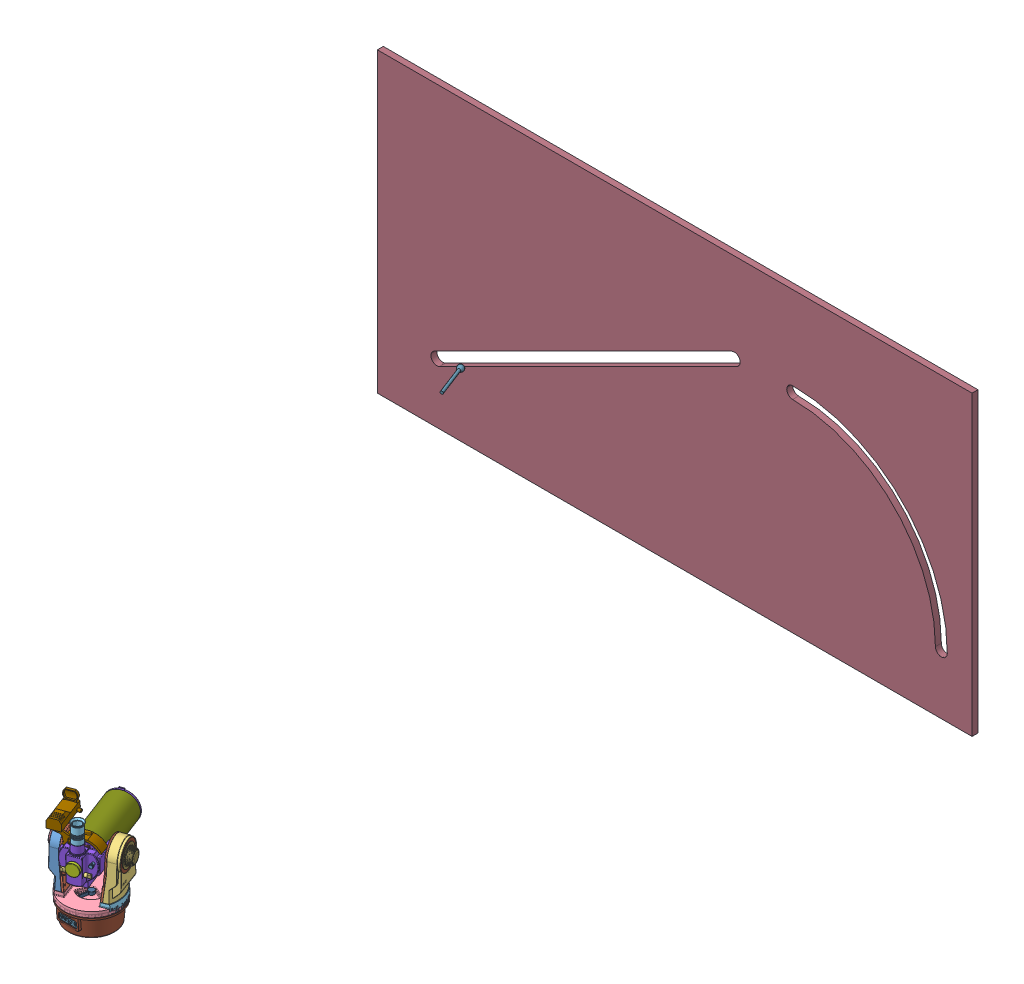
SolidWorks assembly meade, configuration Défaut. Lengths in mm.
Overall size (2000 1013.54 2177.52).
169 component instances, 90 part files, 14 mates.
Components (placement in the parent):
- fourche-1: fourche [Défaut] at (-625.4389 13.0791 -499.8104) x (-0.957342 -0.017413 0.288434) z (-0.288497 0.001172 -0.95748) size (198.85 238.33 188.61)
  - branche equilibrage-1: branche equilibrage [Défaut] at (-444.0293 45.9192 -837.0232) x (0.999848 0.017413 0.00001) z (0.00001 -0.001172 0.999999) size (42.16 177.75 110.07)
  - Plaque carter équilibrage-1: Plaque carter équilibrage [Défaut] at (-443.0317 45.9366 -837.0903) x (0.999848 0.017413 0.00001) z (0.00001 -0.001172 0.999999) size (27.56 165.18 109.18)
  - Plaque carter équilibrage-2: Plaque carter équilibrage [Défaut] at (-468.0617 45.0668 -480.7137) x (-0.999848 -0.017413 -0.00001) z (-0.00001 0.001172 -0.999999) size (27.56 165.18 109.18)
  - branche motorisée-1: branche motorisée [Défaut] at (-441.716 45.9434 -837.1795) x (0.999848 0.017413 0.00001) z (0.00001 -0.001172 0.999999) size (49.59 177.72 110.04)
  - PIED DE fourche-1: PIED DE fourche [Défaut] at (-454.4692 -14.4541 -658.8869) x (0.999848 0.017413 0.00001) z (0.00001 -0.001172 0.999999) size (191.94 35.1 188.57)
    - Pied de fourche-1: Pied de fourche [Défaut] at (12.1809 59.9857 -178.2534) size (191.94 35.1 188.57)
    - Pied de fourche1-1: Pied de fourche1 [Défaut] at (-12.1809 59.9857 178.0188) x (-1 0 0) z (0 0 -1) size (54.8 35.1 115.86)
  - rondelle vis m8_50-1: rondelle vis m8_50 [Défaut] at (-454.2843 -25.0712 -659.0167) x (0.997592 0.017452 -0.067129) z (0.017413 -0.999848 -0.001172) size (26.8 26.16 7)
  - VisHM8_50-1: VisHM8_50 [Défaut] at (-454.3818 -19.4721 -659.0102) x (0.997592 0.017452 -0.067129) z (0.017413 -0.999848 -0.001172) size (12.6 14.55 55.47)
  - limiteur de couple embase-1: limiteur de couple embase [Défaut] at (-453.5008 -70.0544 -659.0694) x (0.06714 0 0.997744) z (-0.997592 -0.017452 0.067129) size (25.3 5 25.3)
  - Roue à denture hélicoïdale m=0,5 Z=60-1: Roue à denture hélicoïdale m=0,5 Z=60 [Défaut] at (-453.6431 -61.8856 -659.0599) x (0.201032 0.002353 0.979582) z (-0.017413 0.999848 0.001172) size (31.07 31.07 6.34)
  - Levier de débrayage-1: Levier de débrayage [Défaut] at (-491.4971 43.1006 -833.8173) x (0.963244 0.01709 -0.268082) z (0.268062 0.003539 0.963395) size (36.12 10 38.96)
  - plateau-1: plateau [Défaut] at (-454.3861 -19.2221 -659.0099) x (-0.997592 -0.017452 0.067129) z (0.017413 -0.999848 -0.001172) size (170 170 47)
  - EcrouHM 20-2: EcrouHM 20 [Défaut] at (-453.9456 -44.5183 -659.0395) x (0.06714 0 0.997744) z (-0.017413 0.999848 0.001172) size (30 34.64 12)
  - motoreducteur fourche-1: motoreducteur fourche [Défaut] at (-542.1299 45.8782 -641.824) x (0.06714 0 0.997744) z (0.997592 0.017452 -0.067129) size (70.5 139.71 33.06)
    - rep. 01 pignon arbre moteur + disque-1: rep. 01 pignon arbre moteur + disque [Défaut] at (0 -0.36 0) size (19 10.8 19)
    - rep. 02-03 roue Z56-1: rep. 02-03 roue Z56 [Défaut] at (0.8779 -0.6486 0.8082) x (0.995701 0 0.092628) z (-0.092628 0 0.995701) size (28.76 10.95 28.76)
    - rep. 08-09 roue inter-1: rep. 08-09 roue inter [Défaut] at (-0.15 -0.2381 0) x (1 0 0) z (0 0 1) size (12.96 5.74 12.96)
    - rep. 06-07 roue inter-1: rep. 06-07 roue inter [Défaut] at (-0.15 -0.0981 0) x (1 0 0) z (0 0 1) size (13 5.74 13)
    - rep. 04-05 roue inter-1: rep. 04-05 roue inter [Défaut] at (-21.6079 -0.6386 5.1059) x (0.907401 0 -0.420265) z (0.420265 0 0.907401) size (13 5.74 13)
    - bati-1: bati [Défaut] at (103.3128 129.885 -87.3106) size (70.5 138.91 24)
      - Axe Rep19bis-1: Axe Rep19bis [Défaut] at (-92.1856 -130.245 98.2871) x (-0.137137 0 0.990552) z (-0.990552 0 -0.137137) size (3 14 3)
      - moteur-1: moteur [Défaut] at (-103.3128 -129.885 87.3106) size (18 46.5 24)
      - axe-1: axe [Défaut] at (-111.605 -120.0821 97.7106) x (0.934599 0 -0.355704) z (0 -1 0) size (3 3 39)
      - bati2-1: bati2 [Défaut] at (-77.4849 -277.8736 138.6581) x (1 0 0) z (0 0 -1) size (17.4 55.11 17.4)
        - rondelle alu-1: rondelle alu [Défaut] at (-55.9783 -35.2009 30.6529) size (17.4 2.5 17.4)
        - Rondelle M6_1-1: Rondelle M6_1 [Défaut] at (-55.9783 -35.2009 30.6529) size (16.67 2.55 16.67)
        - rondelle alu_1-1: rondelle alu_1 [Défaut] at (-55.9783 -35.2009 30.6529) size (17.4 2.5 17.4)
        - Entretoise_1-1: Entretoise_1 [Défaut] at (-55.9783 -35.2009 30.6529) size (16.5 6 16.5)
        - Entretoise-1: Entretoise [Défaut] at (-55.9783 -35.2009 30.6529) size (16.5 6 16.5)
        - Rondelle M6-1: Rondelle M6 [Défaut] at (-55.9783 -35.2009 30.6529) size (16.67 2.55 16.67)
        - rep. 16 Ecrou M6-1: rep. 16 Ecrou M6 [Défaut] at (18.5294 -120.4752 48.0628) x (-0.896454 0 -0.443136) z (-0.443136 0 0.896454) size (12.68 6 11.39)
      - corps1-1: corps1 [Défaut] at (-126.5989 -147.7633 97.7106) size (62.7 74.5 12)
      - corps2-1: corps2 [Défaut] at (-126.5989 -147.7633 85.7106) size (62.7 50 12)
      - châpe en alu-1: châpe en alu [Défaut] at (-133.4632 -157.3984 87.2051) size (33.3 38 19.61)
    - vis-1: vis [Défaut] at (7.3554 -71.4832 9.6533) x (1 0 0) z (0 1 0) size (33.09 33.06 82.71)
      - Vis san fin m=0,5 - 1 filet(s)-2: Vis san fin m=0,5 - 1 filet(s) [Défaut] at (-0.6479 -0.6412 0.3804) x (0.7262 -0.687484 0) z (0 0 1) size (8.16 8.16 68.9)
      - rep12-4: rep12 [Défaut] at (-11.6724 36.0347 43.7266) x (0.537117 -0.843508 0) z (-0.843508 -0.537117 0) size (23.91 29.81 24)
    - engrenage-1: engrenage [Défaut] at (-45.9983 -125.8694 31.0757) x (-0.919401 0 0.393321) z (0.393321 0 0.919401) size (12.99 17.44 12.99)
      - rep.11SLDPRT-1: rep.11SLDPRT [Défaut] at (-64.557 -106.8565 -14.5787) size (9.52 16 9.52)
      - rep. yacine-1: rep. yacine [Défaut] at (-64.557 -106.8565 -14.5787) size (12.99 1.44 12.99)
    - Vis à tête cylindrique à six pans creux Chc M2,5 - 8-1: Vis à tête cylindrique à six pans creux Chc M2,5 - 8 [Défaut] at (6.7074 -20.6971 10.2945) x (0.636786 0 0.771041) z (0 -1 0) size (4.2 4.2 10.57)
    - joint 9 5 emb-1: joint 9 5 emb [Défaut] at (6.7074 -89.1506 10.2945) size (13.5 2 13.5)
    - joint 9 5 emb-2: joint 9 5 emb [Défaut] at (6.7074 -53.1506 10.2945) size (13.5 2 13.5)
  - Vis sans tête à six pans creux à bout cuvette M3 - 3-1: Vis sans tête à six pans creux à bout cuvette M3 - 3 [Réaliste] at (-445.1418 -17.1499 -659.6319) x (-0.019293 -0.859815 -0.51024) z (0.066624 -0.510307 0.857408) size (3.03 3.08 3.04)
  - Vis à tête cylindrique bombée cruciforme type H M3 - 10-1: Vis à tête cylindrique bombée cruciforme type H M3 - 10 [Filetage Réaliste] at (-521.841 56.7793 -695.504) x (-0.997592 -0.017452 0.067129) z (-0.0364 0.955572 -0.292501) size (12.58 5.6 5.6)
  - Vis à tête cylindrique bombée cruciforme type H M3 - 10-2: Vis à tête cylindrique bombée cruciforme type H M3 - 10 [Filetage Réaliste] at (-508.9533 16.8988 -611.179) x (-0.997592 -0.017452 0.067129) z (-0.040277 -0.642181 -0.765494) size (12.58 5.6 5.6)
  - Vis à tête cylindrique bombée cruciforme type H M3 - 10-3: Vis à tête cylindrique bombée cruciforme type H M3 - 10 [Filetage Réaliste] at (-514.8616 16.8988 -698.9804) x (-0.997592 -0.017452 0.067129) z (-0.068087 0.06176 -0.995766) size (12.58 5.6 5.6)
  - Vis à tête cylindrique bombée cruciforme type H M3 - 10-4: Vis à tête cylindrique bombée cruciforme type H M3 - 10 [Filetage Réaliste] at (-521.2936 154.7556 -654.4481) x (-0.997592 -0.017452 0.067129) z (-0.06714 0 -0.997744) size (12.58 5.6 5.6)
  - Vis à tête cylindrique bombée cruciforme type H M3 - 10-5: Vis à tête cylindrique bombée cruciforme type H M3 - 10 [Filetage Réaliste] at (-516.3356 56.7793 -613.689) x (-0.997592 -0.017452 0.067129) z (-0.06714 0 -0.997744) size (12.58 5.6 5.6)
  - Vis à tête cylindrique bombée cruciforme type H M3 - 10-7: Vis à tête cylindrique bombée cruciforme type H M3 - 10 [Filetage Réaliste] at (-393.6444 157.0051 -663.0973) x (0.997592 0.017452 -0.067129) z (0.06714 0 0.997744) size (12.58 5.6 5.6)
  - Vis à tête cylindrique bombée cruciforme type H M3 - 10-8: Vis à tête cylindrique bombée cruciforme type H M3 - 10 [Filetage Réaliste] at (-401.1787 18.9039 -706.6898) x (0.997592 0.017452 -0.067129) z (0.06714 0 0.997744) size (12.58 5.6 5.6)
  - Vis à tête cylindrique bombée cruciforme type H M3 - 10-10: Vis à tête cylindrique bombée cruciforme type H M3 - 10 [Filetage Réaliste] at (-395.1895 59.0113 -704.086) x (0.997592 0.017452 -0.067129) z (0.06714 0 0.997744) size (12.58 5.6 5.6)
  - Vis à tête cylindrique fendue CS M4 - 10-1: Vis à tête cylindrique fendue CS M4 - 10 [Défaut] at (-539.7157 125.5672 -628.3483) x (0.067415 -0.016315 0.997592) z (-0.997592 -0.017452 0.067129) size (7 7 10.62)
  - Vis à tête cylindrique fendue CS M4 - 10-2: Vis à tête cylindrique fendue CS M4 - 10 [Défaut] at (-538.2089 116.0774 -615.8713) x (0.067415 -0.016315 0.997592) z (-0.997592 -0.017452 0.067129) size (7 7 10.62)
  - Vis à tête cylindrique fendue CS M4 - 10-3: Vis à tête cylindrique fendue CS M4 - 10 [Défaut] at (-539.3849 106.5701 -628.3705) x (0.067415 -0.016315 0.997592) z (-0.997592 -0.017452 0.067129) size (7 7 10.62)
  - Vis à tête cylindrique bombée cruciforme type H M3 - 12-2: Vis à tête cylindrique bombée cruciforme type H M3 - 12 [Filetage Réaliste] at (-395.2704 18.9039 -618.8883) x (0.997592 0.017452 -0.067129) z (0.067129 0.000586 0.997744) size (14.59 5.6 5.6)
  - Vis à tête cylindrique bombée cruciforme type H M3 - 12-3: Vis à tête cylindrique bombée cruciforme type H M3 - 12 [Filetage Réaliste] at (-389.684 59.0113 -622.271) x (0.997592 0.017452 -0.067129) z (0.068185 -0.42423 0.902984) size (14.59 5.6 5.6)
  - Vis à tête cylindrique bombée cruciforme type H M3 - 25-1: Vis à tête cylindrique bombée cruciforme type H M3 - 25 [Filetage Réaliste] at (-516.5693 58.6063 -628.1014) x (-0.997592 -0.017452 0.067129) z (-0.067129 0.486457 -0.871122) size (32.61 5.6 5.6)
  - Vis à tête cylindrique bombée cruciforme type H M3 - 25-2: Vis à tête cylindrique bombée cruciforme type H M3 - 25 [Filetage Réaliste] at (-520.3322 72.7741 -680.3366) x (-0.997592 -0.017452 0.067129) z (-0.067129 0.486457 -0.871122) size (32.61 5.6 5.6)
  - Vis à tête cylindrique bombée cruciforme type H M3 - 25-3: Vis à tête cylindrique bombée cruciforme type H M3 - 25 [Filetage Réaliste] at (-519.8272 43.7786 -680.3706) x (-0.997592 -0.017452 0.067129) z (0.067053 0.00493 0.997737) size (32.61 5.6 5.6)
  - Vis à tête cylindrique bombée cruciforme type H M3 - 20-1: Vis à tête cylindrique bombée cruciforme type H M3 - 20 [Filetage Réaliste] at (-531.1265 -25.9655 -653.8459) x (-0.017413 0.999848 0.001172) z (0.998816 0.017342 0.045444) size (22.61 5.6 5.6)
  - Vis à tête cylindrique bombée cruciforme type H M3 - 20-2: Vis à tête cylindrique bombée cruciforme type H M3 - 20 [Filetage Réaliste] at (-512.8439 -25.695 -612.9812) x (-0.017413 0.999848 0.001172) z (0.998816 0.017342 0.045444) size (22.61 5.6 5.6)
  - Vis à tête cylindrique bombée cruciforme type H M3 - 20-3: Vis à tête cylindrique bombée cruciforme type H M3 - 20 [Filetage Réaliste] at (-517.7505 -25.6821 -696.841) x (-0.017413 0.999848 0.001172) z (0.998816 0.017342 0.045444) size (22.61 5.6 5.6)
  - Vis à tête cylindrique bombée cruciforme type H M3 - 20-4: Vis à tête cylindrique bombée cruciforme type H M3 - 20 [Filetage Réaliste] at (-395.7403 -23.5476 -705.0512) x (-0.017413 0.999848 0.001172) z (0.998816 0.017342 0.045444) size (22.61 5.6 5.6)
  - Vis à tête cylindrique bombée cruciforme type H M3 - 20-5: Vis à tête cylindrique bombée cruciforme type H M3 - 20 [Filetage Réaliste] at (-377.4577 -23.2771 -664.1865) x (-0.017413 0.999848 0.001172) z (0.998816 0.017342 0.045444) size (22.61 5.6 5.6)
  - Vis à tête cylindrique bombée cruciforme type H M3 - 20-6: Vis à tête cylindrique bombée cruciforme type H M3 - 20 [Filetage Réaliste] at (-390.8337 -23.5604 -621.1914) x (-0.017413 0.999848 0.001172) z (0.998816 0.017342 0.045444) size (22.61 5.6 5.6)
- tube-1: tube [Défaut] at (-0.2356 70.625 -0.6263) x (-0.935954 0 0.352121) z (-0.352104 0.009923 -0.935908) size (229.47 195.18 484.9)
  - Capuchon port photo-2: Capuchon port photo [Défaut] at (20.0265 52.1414 -183.8549) x (0.753442 -0.654583 0.06202) z (-0.29492 -0.252137 0.921656) size (39.95 39.82 23.78)
  - support objectif-2: support objectif [Défaut] at (0 67.5 -76) size (179.88 130.77 134.7)
  - Palier d'embrayage-2: Palier d'embrayage [Défaut] at (24.7034 252.6163 -72.3954) x (0.997744 -0.06714 0) z (-0.06714 -0.997744 0) size (14.91 34.8 28.76)
  - palier-2: palier [Défaut] at (-93.6662 67.5 0) x (1 0 0) z (0 -0.589029 0.808112) size (10.05 25.5 25.5)
  - Roue à denture hélicoïdale m=0,5 Z=60-3: Roue à denture hélicoïdale m=0,5 Z=60 [Défaut] at (-77.15 67.5 0) x (0 0.783284 -0.621664) z (1 0 0) size (31.07 31.07 6.34)
  - Plaque repérage angulaire-3: Plaque repérage angulaire [Défaut] at (-159.1429 162.8547 -174.0321) x (0.997744 -0.051519 0.043053) z (-0.06714 -0.765605 0.639798) size (6.77 89 88.85)
  - molette blocage vertical-2: molette blocage vertical [Défaut] at (25.2373 156.4775 -169.1848) x (0.997744 -0.051429 0.043161) z (-0.06714 -0.764265 0.641398) size (31.87 70 69.98)
  - molette blocage 2 vertical-2: molette blocage 2 vertical [Défaut] at (-32.8172 155.1442 169.8822) x (-0.997741 -0.051084 -0.043619) z (0.067172 -0.759198 -0.647384) size (27.85 70 69.98)
  - Plaque repérage angulaire-4: Plaque repérage angulaire [Défaut] at (151.5627 161.1167 174.9858) x (-0.997741 -0.051084 -0.043619) z (0.067172 -0.759198 -0.647384) size (6.77 89 88.85)
  - Embout fileté-2: Embout fileté [Défaut] at (31.1097 71.2083 -217.7977) x (0.995668 0.069272 0.06202) z (-0.030498 -0.386808 0.921656) size (96.08 90.33 41.21)
  - miroir-2: miroir [Défaut] at (1.5401 49.2079 -414.2886) x (0 -0.998075 0.06202) z (-0.383759 0.057271 0.921656) size (89.51 86.43 44.67)
  - tube-2: tube [Défaut] at (0 67.5 -53.7618) x (0 0 -1) z (1 0 0) size (225 100 100)
  - menisque-2: menisque [Défaut] at (-10.827 126.3859 145.8849) x (-0.376431 0.924349 0.062271) z (0.377105 0.091483 0.921641) size (110.67 106.16 46.27)
    - menisque-1: menisque [Défaut] at (-56.116 -127.6725 -342.9742) size (27.57 28.77 19.69)
    - Piece1-1: Piece1 [Défaut] at (-57.8098 16.1933 3.3103) x (0.972599 -0.230535 0.030091) z (-0.028457 0.010411 0.999541) size (92 86.87 40.19)
  - molette-2: molette [Défaut] at (16.1783 77.4199 -201.1536) x (0.997152 -0.042906 0.06202) z (-0.073715 -0.380942 0.921656) size (12.27 29.01 54.01)
  - Vis porte oculaire-2: Vis porte oculaire [Défaut] at (70.5773 71.9334 3.0696) x (0.833291 0.517003 -0.195792) z (-0.515568 0.854579 0.062325) size (15.46 8.19 13.39)
  - bouton miroir-3: bouton miroir [Défaut] at (118.3372 40.7094 -82.3) x (0.999979 -0.006557 0) z (0 0 1) size (83.58 43.34 43.14)
    - bouton miroir-1: bouton miroir [Défaut] at (-90.8002 18.3233 -120.2299) x (0.996615 -0.012919 0.081184) z (-0.081184 -0.309873 0.947306) size (41.27 12.61 13.28)
    - bouton miroir-2: bouton miroir [Défaut] at (-145.9581 -6.2943 -120.2299) x (-0.996615 0.012919 0.081184) z (0.081184 0.309873 0.947306) size (41.27 12.61 13.28)
    - petit miroir-1: petit miroir [Défaut] at (-118.5103 26.0141 2.75) x (0.999979 0.006557 0) z (0.004637 -0.707092 0.707107) size (30 26.01 35)
  - oculaire-2: oculaire [Défaut] at (0 149.5136 -0.7045) x (0 0 1) z (-1 0 0) size (38 81.5 38)
    - oculaire-1: oculaire [Défaut] at (-78.8455 -41.743 0) size (38 81.5 38)
    - lentille-1: lentille [Défaut] at (-81.1151 5.0064 0) x (0 -1 0) z (0 0 1) size (10.53 25 25)
      - lentille 1-1: lentille 1 [Défaut] at (-6.7507 2.2696 0) size (8.01 25 25)
      - lentille 2-1: lentille 2 [Défaut] at (-12.7507 2.2696 0) size (4.52 25 25)
    - lentille-2: lentille [Défaut] at (-76.963 10.0077 1.2678) x (0 1 0) z (-0.558618 0 0.829425) size (10.53 25 25)
      - lentille 1-1: lentille 1 [Défaut] at (-6.7507 2.2696 0) size (8.01 25 25)
      - lentille 2-1: lentille 2 [Défaut] at (-12.7507 2.2696 0) size (4.52 25 25)
  - faisceau2-2: faisceau2 [Défaut] at (0 78.827 -14.9477) x (0 0 -1) z (1 0 0) size (437.42 120.49 0.34) (hidden)
  - fleche-13: fleche [Défaut] at (0 108.7031 110.8339) x (0 0 1) z (-0.886861 -0.462037 0) size (8 5.6 5.6) (hidden)
  - fleche-14: fleche [Défaut] at (0 88.228 83.446) x (0 0.178036 -0.984024) z (1 -0.000403 -0.000073) size (8 5.6 5.6) (hidden)
  - fleche-15: fleche [Défaut] at (0 75.6322 94.3005) x (0 0.005533 0.999985) z (0.072331 0.997365 -0.005519) size (8 5.6 5.6) (hidden)
  - fleche-16: fleche [Défaut] at (0 108.7103 294.2676) x (0 0.017452 0.999848) z (-0.523715 0.851763 -0.014868) size (8 5.6 5.6) (hidden)
  - fleche-17: fleche [Défaut] at (0 127.4306 -74.061) x (0 -0.974863 -0.222804) z (-0.735553 0.150943 -0.660438) size (8 5.6 5.6) (hidden)
  - fleche-18: fleche [Défaut] at (0 183.519 -69.8214) x (0 -1 0) z (-0.316126 0 0.948717) size (8 5.6 5.6) (hidden)
  - faisceau1-2: faisceau1 [Défaut] at (0 -20.7845 -6.8996) x (0 0 -1) z (1 0 0) size (447.26 167.74 0.41) (hidden)
  - fleche-19: fleche [Défaut] at (0 30.6251 284.852) x (0 0 1) z (-0.426184 0.904636 0) size (8 5.6 5.6) (hidden)
  - fleche-20: fleche [Défaut] at (0 27.6512 105.4051) x (0 0 1) z (-0.740163 -0.672427 0) size (8 5.6 5.6) (hidden)
  - fleche-21: fleche [Défaut] at (0 46.7601 79.6116) x (0 -0.171906 -0.985113) z (0.984293 0.173915 -0.030349) size (8 5.6 5.6) (hidden)
  - fleche-22: fleche [Défaut] at (0 59.5724 94.0494) x (0 -0.005145 0.999987) z (-0.101559 -0.994816 -0.005119) size (8 5.6 5.6) (hidden)
  - fleche-23: fleche [Défaut] at (0 127.1897 -84.7907) x (0 -0.982309 0.187268) z (-0.405585 0.171174 0.897887) size (8 5.6 5.6) (hidden)
  - fleche-24: fleche [Défaut] at (0 183.4575 -88.3366) x (0 -1 0) z (-0.976187 0 0.216931) size (8 5.6 5.6) (hidden)
  - cache-2: cache [Défaut] at (0 67.5 174.5) x (0 0 -1) z (1 0 0) size (10 111 100)
  - Module LNT-2: Module LNT [Défaut] at (0 67.5 -16) x (0.999806 -0.019718 0) z (0 0 1) size (140.9 99.11 110)
  - Vis à tête cylindrique fendue CS M3 - 10-1: Vis à tête cylindrique fendue CS M3 - 10 [Défaut] at (27 106.7707 -61.5) size (5.5 5.5 12.01)
- CARTER EMBASE-2: CARTER EMBASE [Défaut] at (-38.5593 -33.7526 0) x (-1 0 0) z (0 0 -1) size (2000 1017.04 2124.41)
  - Carter embase-1: Carter embase [Défaut] at (-38.5593 34.3526 0) size (182.1 77.5 182)
  - palier-1: palier [Défaut] at (-38.7022 18.1339 0.128) x (-0.744983 0 0.667084) z (0.667084 0 0.744983) size (45.68 15.3 45.68)
    - palier alu-1: palier alu [Défaut] at (-0.1919 7.7813 0) size (40 13.5 40)
    - palier axial-1: palier axial [Défaut] at (-0.1919 -6.6187 0) size (33 6.3 33)
    - palier axial-2: palier axial [Défaut] at (-0.1919 8.6813 0) x (-0.837169 0 -0.546944) z (-0.546944 0 0.837169) size (33 6.3 33)
  - plaque branchement-1: plaque branchement [Défaut] at (-38.5593 -18.7385 -76.5024) x (1 0 0) z (0 0.068841 0.997628) size (62.31 43.19 20.2)
  - carter couvercle-1: carter couvercle [Défaut] at (-38.5593 -43.1474 0) x (0 0 1) z (-1 0 0) size (145 23 145) (hidden)
  - anneau guide-1: anneau guide [Défaut] at (-38.5593 19.8526 0) x (-0.683843 0 0.729629) z (0 1 0) size (46.6 56.5 4.2)
  - support palier-1: support palier [Défaut] at (-38.5593 58.1532 0) x (0.258819 0 -0.965926) z (0.965926 0 0.258819) size (170.5 70.67 170.49)
  - reducteur embase-1: reducteur embase [Défaut] at (-74.9499 2.4826 -18.0358) x (0 0 1) z (0 -1 0) size (101.77 85.1 39.66)
    - rep. 01 pignon arbre moteur + disque-1: rep. 01 pignon arbre moteur + disque [Défaut] at (0.9543 -1.36 18.0797) x (0.78085 0 0.624719) z (-0.624719 0 0.78085) size (19 10.8 19)
    - rep. 02-03 roue Z56-1: rep. 02-03 roue Z56 [Défaut] at (-12.7174 -0.5 -2.1104) x (0.531735 0 -0.846911) z (0.846911 0 0.531735) size (28.76 10.95 28.76)
    - rep. 08-09 roue inter-1: rep. 08-09 roue inter [Défaut] at (-2.3943 -0.3381 0.4364) x (0.975998 0 -0.217777) z (0.217777 0 0.975998) size (12.96 5.74 12.96)
    - rep. 06-07 roue inter-1: rep. 06-07 roue inter [Défaut] at (-3.1771 0.3019 0.7148) x (0.955582 0 -0.294727) z (0.294727 0 0.955582) size (13 5.74 13)
    - roue rep 12 (petite folle)-1: roue rep 12 (petite folle) [Défaut] at (0.2679 -0.4 -0.3808) x (0.999222 0 0.039446) z (-0.039446 0 0.999222) size (13 3.24 13)
    - rep. 04-05 roue inter-1: rep. 04-05 roue inter [Défaut] at (2.2907 -0.16 -1.8606) x (0.977065 0 0.21294) z (-0.21294 0 0.977065) size (13 5.74 13)
    - bati emb-1: bati emb [Défaut] at (103.3128 129.885 -87.3106) size (101.77 84.35 25.96)
      - coque droite emb-1: coque droite emb [Défaut] at (-103.3128 -129.885 87.3106) size (93.29 54 12.58)
      - Axe Rep19bis emb-1: Axe Rep19bis emb [Défaut] at (-103.9752 -130.143 87.3656) x (0.998781 0 -0.049366) z (0.049366 0 0.998781) size (3 15.3 3)
      - Axe Rep20.bis emb-1: Axe Rep20.bis emb [Défaut] at (-97.8983 -130.0094 79.9317) x (0.927514 0 0.373788) z (-0.373788 0 0.927514) size (3 22 3)
      - coque gauche emb-1: coque gauche emb [Défaut] at (-103.3128 -129.885 87.3106) size (94.76 55 11.51)
      - axe emb-1: axe emb [Défaut] at (-111.605 -119.0221 97.7106) x (0.824702 0 -0.565567) z (0 -1 0) size (3 3 15)
      - Axe Rep19bis emb-2: Axe Rep19bis emb [Défaut] at (-101.4828 -129.945 90.8669) x (0.715658 0 -0.698451) z (0.698451 0 0.715658) size (3 15.3 3)
      - moteur-2: moteur [Défaut] at (-103.3128 -129.885 87.3106) size (18 46.5 24)
      - châpe en alu emb-2: châpe en alu emb [Défaut] at (-103.4628 -123.4884 87.3106) size (32 38 21)
      - Entretoise emb-3: Entretoise emb [Défaut] at (-100.6729 -123.5884 80.7498) x (0.982912 0 0.184074) z (-0.184074 0 0.982912) size (17.65 5.7 17.65)
      - rondelle alu emb-3: rondelle alu emb [Défaut] at (-90.9589 -123.8884 68.1548) x (0.821605 0 0.570058) z (-0.570058 0 0.821605) size (17.4 2.65 17.4)
      - rep. 16 Ecrou M6 emb-2: rep. 16 Ecrou M6 emb [Défaut] at (-102.7157 -122.485 84.9564) x (0.99792 0 0.06446) z (-0.06446 0 0.99792) size (12.68 6 11.39)
      - Rondelle M6 emb-2: Rondelle M6 emb [Défaut] at (-94.2052 -123.7384 71.161) x (0.88187 0 0.471493) z (-0.471493 0 0.88187) size (16 1.8 16)
      - joint 9 5 emb-3: joint 9 5 emb [Défaut] at (-66.605 -149.1255 97.7106) size (13.5 2 13.5)
      - joint 9 5 emb-4: joint 9 5 emb [Défaut] at (-66.605 -183.1255 97.7106) x (0.837169 0 0.546944) z (0.546944 0 -0.837169) size (13.5 2 13.5)
      - rondelle alu emb-4: rondelle alu emb [Défaut] at (-91.5165 -167.7384 68.6232) x (0.832295 0 0.554332) z (-0.554332 0 0.832295) size (17.4 2.65 17.4)
      - Entretoise emb-4: Entretoise emb [Défaut] at (-30.2975 -208.6627 109.115) x (-0.835834 0 -0.548983) z (-0.548983 0 0.835834) size (17.65 5.7 17.65)
      - Rondelle M6 emb-3: Rondelle M6 emb [Défaut] at (-29.9622 -208.5127 109.2274) x (-0.837169 0 -0.546944) z (-0.546944 0 0.837169) size (16 1.8 16)
      - Vis à tête cylindrique bombée cruciforme type H M3 - 12-1: Vis à tête cylindrique bombée cruciforme type H M3 - 12 [Filetage Réaliste] at (-110.205 -142.8221 109.7106) x (0 0 -1) z (1 0 0) size (14.59 5.6 5.6)
      - Vis à tête cylindrique bombée cruciforme type H M3 - 12-2: Vis à tête cylindrique bombée cruciforme type H M3 - 12 [Filetage Réaliste] at (-93.3519 -120.1721 111.5106) x (0 0 -1) z (-0.592827 0.80533 0) size (14.59 5.6 5.6)
    - vis emb-1: vis emb [Défaut] at (37.3558 -36.1406 9.7588) x (1 0 0) z (0 1 0) size (25.74 25.82 76.16)
      - Vis san fin m=0,5 - 1 filet(s) emb-1: Vis san fin m=0,5 - 1 filet(s) emb [Défaut] at (-0.6479 -0.6412 0) size (8.16 8.16 68.9)
      - rep12 emb-3: rep12 emb [Défaut] at (-38.2155 6.7975 36.7974) x (0.996839 0.079451 0) z (0.079451 -0.996839 0) size (23.91 23.8 24)
    - engrenage-1: engrenage [Défaut] at (64.1683 106.4565 3.5924) x (0.967334 0 -0.253504) z (0.253504 0 0.967334) size (12.99 17.44 12.99)
      - rep.11SLDPRT-1: rep.11SLDPRT [Défaut] at (-64.557 -106.8565 -14.5787) size (9.52 16 9.52)
      - rep. yacine-1: rep. yacine [Défaut] at (-64.557 -106.8565 -14.5787) size (12.99 1.44 12.99)
    - Vis à tête cylindrique à six pans creux Chc M2,5 - 8-1: Vis à tête cylindrique à six pans creux Chc M2,5 - 8 [Défaut] at (36.7078 7.7163 10.4) x (1 0 0) z (0 -1 0) size (4.2 4.2 10.57)
  - Vis à tête fraisée FS M5 - 16-1: Vis à tête fraisée FS M5 - 16 [Défaut] at (-102.5593 -40.456 0) x (-1 0 0) z (0 1 0) size (10.32 10.4 16)
  - Vis à tête fraisée FS M5 - 16-2: Vis à tête fraisée FS M5 - 16 [Défaut] at (-6.5593 -40.456 55.4256) x (0.5 0 0.866025) z (0 1 0) size (10.32 10.4 16)
  - Vis à tête fraisée FS M5 - 16-3: Vis à tête fraisée FS M5 - 16 [Défaut] at (-6.5593 -40.456 -55.4256) x (0.5 0 -0.866025) z (0 1 0) size (10.32 10.4 16)
  - Vis à tête cylindrique bombée cruciforme type H M3 - 12-1: Vis à tête cylindrique bombée cruciforme type H M3 - 12 [Filetage Réaliste] at (-58.5127 -18.1174 -56.178) x (0 1 0) z (0 0 1) size (14.59 5.6 5.6)
  - Vis à tête cylindrique bombée cruciforme type H M3 - 12-2: Vis à tête cylindrique bombée cruciforme type H M3 - 12 [Filetage Réaliste] at (-89.2627 -18.7174 28.322) x (0 1 0) z (0 0 1) size (14.59 5.6 5.6)
  - Vis à tête cylindrique fendue CS M4 - 10-1: Vis à tête cylindrique fendue CS M4 - 10 [Défaut] at (-38.4593 -1.6174 37.562) x (1 0 0) z (0 1 0) size (7 7 10.62)
  - Vis à tête cylindrique fendue CS M4 - 10-2: Vis à tête cylindrique fendue CS M4 - 10 [Défaut] at (-31.0593 -0.5174 24.912) x (1 0 0) z (0 1 0) size (7 7 10.62)
  - Vis à tête cylindrique fendue CS M4 - 10-3: Vis à tête cylindrique fendue CS M4 - 10 [Défaut] at (-45.8593 -0.5174 24.912) x (1 0 0) z (0 1 0) size (7 7 10.62)
  - tableau-1: tableau [Défaut] at (-1000 -29.6111 2020) x (1 0 0) z (0 1 0) size (2000 20 1000)
- Cible-1: Cible [Défaut] at (-710.3262 158.1393 -1888.0781) x (-0.564248 -0.800056 0.203797) z (0.746757 -0.599843 -0.287302) size (20 118.9 20)
Mates (geometry in assembly coordinates):
- Coïncidente76: coincident: line of fourche-1/Roue à denture hélicoïdale m=0,5 Z=60-1 through (0 -90.27 0) axis (0 1 0); plane of ?
- Coïncidente71: coincident anti-aligned: plane of fourche-1/branche motorisée-1; plane of ? through (-85.4162 148.1836 8.0295) normal (-1 0 0)
- Coaxiale7: concentric anti-aligned: cylinder of ? through (-86.4662 138.2317 0.0594) axis (-1 0 0) radius 2.25; circle of fourche-1/Plaque carter équilibrage-2
- Coïncidente51: coincident: point of ?; plane of fourche-1/Plaque carter équilibrage-1 through (24.4187 65.7424 0) normal (0 0 1)
- Coïncidente80: coincident aligned: plane of ? through (0 140.7631 -55.645) normal (1 0 0); plane of assembly through (0 0 0) normal (1 0 0)
- Coïncidente84: coincident anti-aligned: plane of fourche-1/branche motorisée-1 through (79.9459 138.1217 -30.0763) normal (-0.935954 0 0.352121); plane of tube-1/palier-2 through (77.3376 148.4991 -37.0094) normal (0.935954 0 -0.352121)
- Coaxiale10: concentric anti-aligned: cylinder of fourche-1/branche motorisée-1 through (79.9459 138.1217 -30.0763) axis (-0.935954 0 0.352121) radius 12; cylinder of tube-1/palier-2 through (87.6675 138.1217 -32.9813) axis (0.935954 0 -0.352121) radius 12
- Coïncidente91: coincident anti-aligned: plane of CARTER EMBASE-2 through (-38.5593 -33.7526 0) normal (0 0 -1); plane of assembly through (0 0 0) normal (0 0 1)
- Coaxiale14: concentric aligned: cylinder of fourche-1/plateau-1 through (0 1 0) axis (0 1 0) radius 11; cylinder of CARTER EMBASE-2/palier-1/palier axial-1 through (0 -9 0) axis (0 1 0) radius 11.2
- Coïncidente92: coincident anti-aligned: plane of fourche-1/plateau-1 through (35.2719 -9 7.2039) normal (0 -1 0); plane of CARTER EMBASE-2/palier-1/palier axial-1 through (-12.2922 -9 11.0069) normal (0 1 0)
- Coïncidente93: coincident anti-aligned: plane of CARTER EMBASE-2/palier-1/palier axial-2 through (4.2705 -24.3 -15.9378) normal (0 -1 0); plane of fourche-1/EcrouHM 20-2 through (-19.035 -24.3 23.1877) normal (0 1 0)
- Tangent1: tangent: line of CARTER EMBASE-2/tableau-1 through (-829.615 118.7478 -2000) axis (0.894427 0.447214 0); sphere of Cible-1
- Coaxiale15: concentric aligned: cylinder of tube-1/tube-2 through (18.93 137.5882 50.3167) axis (0.352104 -0.009923 0.935908) radius 50; cylinder of Cible-1 through (-710.3262 158.1393 -1888.0781) axis (0.352104 -0.009923 0.935908) radius 4.5565
- Tangent2: tangent anti-aligned: plane of CARTER EMBASE-2/tableau-1 through (961.4407 936.6364 -2000) normal (0 0 1); sphere of Cible-1
